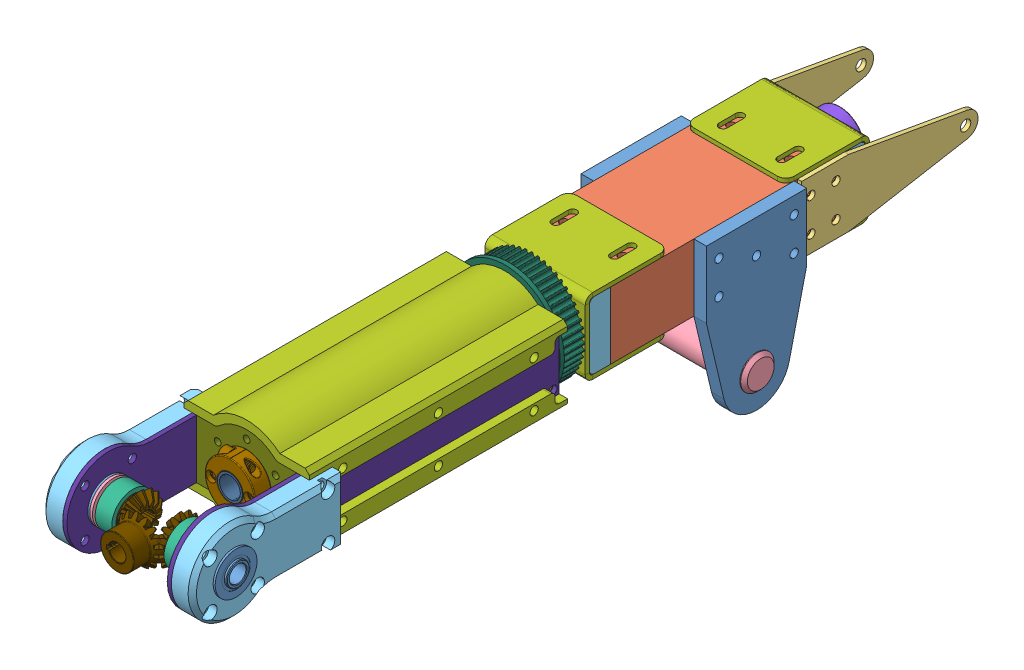
SolidWorks assembly Forearm, configuration Default. Lengths in mm.
Overall size (139.65 143.63 612.78).
45 component instances, 25 part files, 35 mates.
Components (placement in the parent):
- SidePlate^Forearm-1: SidePlate^Forearm [Default] at origin size (47.62 127 76.2) (virtual)
- SidePlate^Forearm-2: SidePlate^Forearm [Default] x (-1 0 0) z (0 0 -1) size (47.62 127 76.2) (virtual)
- Box^Forearm-1: Box^Forearm [Default] at origin size (76.2 50.8 177.8) (virtual)
- BackSidePlate^Forearm-1: BackSidePlate^Forearm [Default] at origin size (41.27 50.8 177.23) (virtual)
- BackSidePlate^Forearm-2: BackSidePlate^Forearm [Default] at (79.375 0 0) size (41.27 50.8 177.23) (virtual)
- 6061K602_HARDENED PRECISION STEEL SHAFT-1: 6061K602_HARDENED PRECISION STEEL SHAFT [6061K602] at (0 609.075 0) size (101.6 25.4 25.4)
- BearingSpacer^Forearm-1: BearingSpacer^Forearm [Default] at origin size (76.2 50.8 22.22) (virtual)
- 6384K367_BALL BEARING-1: 6384K367_BALL BEARING [6384K367] at (0 685.275 115.824) x (1 0 0) z (0 0 -1) size (44.45 44.45 14.3)
- BearingHolder^Forearm-1: BearingHolder^Forearm [Default] at origin size (76.2 57.15 63.5) (virtual)
- BearingSpacer^Forearm-2: BearingSpacer^Forearm [Default] at (0 0 25.4) x (-1 0 0) z (0 0 -1) size (76.2 50.8 22.22) (virtual)
- BearingHolder^Forearm-2: BearingHolder^Forearm [Default] at (0 0 25.4) x (-1 0 0) z (0 0 -1) size (76.2 57.15 63.5) (virtual)
- 6384K367_BALL BEARING-2: 6384K367_BALL BEARING [6384K367] at (0 685.275 -90.424) x (-1 0 0) z (0 0 1) size (44.45 44.45 14.3)
- 6435K160_ONE-PIECE CLAMP-ON SHAFT COLLAR-1: 6435K160_ONE-PIECE CLAMP-ON SHAFT COLLAR [6435K16] at (0 685.275 -104.7242) x (1 0 0) z (0 0 -1) size (38.1 38.11 12.77)
- 9677T100_CLAMP-ON SHAFT COLLAR WITH MOUNTING HOLES-1: 9677T100_CLAMP-ON SHAFT COLLAR WITH MOUNTING HOLES [9677T1] at (0 685.275 159.4517) x (0 -1 0) z (0 0 -1) size (38.14 38.1 13.27)
- 89955K599_Tube^Forearm-1: 89955K599_Tube^Forearm [Default] at origin size (19.05 19.05 463.5) (virtual)
- ThrustBase^Forearm-1: ThrustBase^Forearm [Default] at origin size (44.45 44.45 8.27) (virtual)
- 5909K460_THRUST NEEDLE-ROLLER BEARING-1: 5909K460_THRUST NEEDLE-ROLLER BEARING [5909K46] at (0 685.275 131.2545) x (0 0 -1) z (1 0 0) size (0.81 31.75 31.75)
- 5909K330_THRUST NEEDLE-ROLLER BEARING-1: 5909K330_THRUST NEEDLE-ROLLER BEARING [5909K33] at (0 685.275 132.2467) x (1 0 0) z (0 1 0) size (31.75 1.98 31.75)
- 5909K460_THRUST NEEDLE-ROLLER BEARING-2: 5909K460_THRUST NEEDLE-ROLLER BEARING [5909K46] at (0 685.275 134.0517) x (0 0 -1) z (1 0 0) size (0.81 31.75 31.75)
- PulleySupportPlate^Forearm-1: PulleySupportPlate^Forearm [Default] at origin size (63.5 63.5 3.17) (virtual)
- J4Pulley-1: J4Pulley [Default] at (0 685.275 140.4017) x (-1 0 0) z (0 -1 0) size (84.06 20.68 84.06)
- WristBase^Forearm-1: WristBase^Forearm [Default] at origin size (76.2 63.5 9.53) (virtual)
- WristSidePlate^Forearm-1: WristSidePlate^Forearm [Default] at origin size (3.17 63.5 441.32) (virtual)
- WristSidePlate^Forearm-2: WristSidePlate^Forearm [Default] at (79.375 0 0) size (3.17 63.5 441.32) (virtual)
- WristBase^Forearm-2: WristBase^Forearm [Default] at (0 0 186.6233) size (76.2 63.5 9.53) (virtual)
- 9677T100_CLAMP-ON SHAFT COLLAR WITH MOUNTING HOLES-2: 9677T100_CLAMP-ON SHAFT COLLAR WITH MOUNTING HOLES [9677T1] at (0 685.275 346.075) x (0 -1 0) z (0 0 -1) size (38.14 38.1 13.27)
- 6843K130_MTL MITER GEAR--20 DEG PRESSURE ANGLE-1: 6843K130_MTL MITER GEAR--20 DEG PRESSURE ANGLE [6843K13] at (-31.1638 641.133 394.588) x (0 -0.999847 0.017483) z (0 0.017483 0.999847) size (34.68 21.82 34.5)
- 6843K130_MTL MITER GEAR--20 DEG PRESSURE ANGLE-3: 6843K130_MTL MITER GEAR--20 DEG PRESSURE ANGLE [6843K13] at (-11.812 641.133 437.5638) x (0.017483 -0.999847 0) z (0.999847 0.017483 0) size (34.68 21.82 34.5)
- 6384K361_BALL BEARING-1-1: 6384K361_BALL BEARING-1 [6384K361] at (-41.3385 685.275 406.4) x (0 0 1) z (-1 0 0) size (31.75 31.75 11.13)
- 5909K440_THRUST NEEDLE-ROLLER BEARING-1: 5909K440_THRUST NEEDLE-ROLLER BEARING [5909K44] at (-34.5472 685.275 406.4) size (0.81 23.81 23.81)
- 5909K310_THRUST NEEDLE-ROLLER BEARING-1: 5909K310_THRUST NEEDLE-ROLLER BEARING [5909K31] at (-32.7422 685.275 406.4) x (0 1 0) z (0 0 1) size (23.81 1.98 23.81)
- SideMiterSpacer^Forearm-1: SideMiterSpacer^Forearm [Default] at origin size (2.03 31.75 31.75) (virtual)
- SidePrintedSupport^Forearm-1: SidePrintedSupport^Forearm [Default] at origin size (16.21 63.5 115.89) (virtual)
- 6384K361_BALL BEARING-1-2: 6384K361_BALL BEARING-1 [6384K361] at (-53.9115 685.275 406.4) x (0 0 1) z (1 0 0) size (31.75 31.75 11.13)
- SidePrintedSupport^Forearm-2: SidePrintedSupport^Forearm [Default] at (0 1370.55 0) x (-1 0 0) z (0 0 1) size (16.21 63.5 115.89) (virtual)
- 6384K361_BALL BEARING-1-3: 6384K361_BALL BEARING-1 [6384K361] at (53.9115 685.275 406.4) x (0 0 -1) z (-1 0 0) size (31.75 31.75 11.13)
- 6384K361_BALL BEARING-1-4: 6384K361_BALL BEARING-1 [6384K361] at (41.3385 685.275 406.4) x (0 0 -1) z (1 0 0) size (31.75 31.75 11.13)
- SideMiterSpacer^Forearm-2: SideMiterSpacer^Forearm [Default] at (0 0 812.8) x (-1 0 0) z (0 0 -1) size (2.03 31.75 31.75) (virtual)
- 5909K440_THRUST NEEDLE-ROLLER BEARING-2: 5909K440_THRUST NEEDLE-ROLLER BEARING [5909K44] at (34.5472 685.275 406.4) x (-1 0 0) z (0 0 -1) size (0.81 23.81 23.81)
- 5909K310_THRUST NEEDLE-ROLLER BEARING-2: 5909K310_THRUST NEEDLE-ROLLER BEARING [5909K31] at (32.7422 685.275 406.4) x (0 1 0) z (0 0 1) size (23.81 1.98 23.81)
- 6843K130_MTL MITER GEAR--20 DEG PRESSURE ANGLE-4: 6843K130_MTL MITER GEAR--20 DEG PRESSURE ANGLE [6843K13] at (31.1638 728.9771 393.052) x (0 0.999847 -0.017483) z (0 0.017483 0.999847) size (34.68 21.82 34.5)
- 6391K281_OIL-EMBEDDED SLEEVE BEARING-1: 6391K281_OIL-EMBEDDED SLEEVE BEARING [6391K281] at (-26.162 685.275 406.4) x (0 0 1) z (-1 0 0) size (31.78 31.78 12.7)
- 6391K281_OIL-EMBEDDED SLEEVE BEARING-2: 6391K281_OIL-EMBEDDED SLEEVE BEARING [6391K281] at (26.162 685.275 406.4) x (0 0 1) z (-1 0 0) size (31.78 31.78 12.7)
- WristCover^Forearm-1: WristCover^Forearm [Default] at origin size (95.25 25.4 196.15) (virtual)
- WristCover^Forearm-2: WristCover^Forearm [Default] at (0 1370.55 0) x (-1 0 0) z (0 0 1) size (95.25 25.4 196.15) (virtual)
Mates (geometry in assembly coordinates):
- Concentric1: concentric anti-aligned: cylinder of SidePlate^Forearm-1 through (-47.625 609.075 0) axis (1 0 0) radius 12.7; circle of 6061K602_HARDENED PRECISION STEEL SHAFT-1
- Width1: width anti-aligned: plane of 6061K602_HARDENED PRECISION STEEL SHAFT-1 through (-50.8 609.075 0) normal (-1 0 0); plane of SidePlate^Forearm-2 through (50.8 609.075 0) normal (1 0 0); plane of 6061K602_HARDENED PRECISION STEEL SHAFT-1 through (47.625 609.075 0) normal (1 0 0); plane of SidePlate^Forearm-1 through (-47.625 609.075 0) normal (-1 0 0)
- Concentric2: concentric aligned: cylinder of 6384K367_BALL BEARING-1 through (0 685.275 109.474) axis (0 0 -1) radius 20.6375; cylinder of BearingHolder^Forearm-1 through (0 685.275 120.65) axis (0 0 -1) radius 20.6375
- Coincident2: coincident anti-aligned: plane of 6384K367_BALL BEARING-1 through (0 669.8646 120.65) normal (0 0 -1); plane of BearingHolder^Forearm-1 through (0 0 120.65) normal (0 0 1)
- Concentric3: concentric aligned: cylinder of 6384K367_BALL BEARING-2 through (0 685.275 -84.074) axis (0 0 1) radius 9.525; cylinder of 6435K160_ONE-PIECE CLAMP-ON SHAFT COLLAR-1 through (0 685.275 -111.0742) axis (0 0 1) radius 9.525
- Coincident3: coincident anti-aligned: plane of 6384K367_BALL BEARING-2 through (0 674.4038 -98.3742) normal (0 0 -1); plane of 6435K160_ONE-PIECE CLAMP-ON SHAFT COLLAR-1 through (0 685.275 -98.3742) normal (0 0 1)
- Concentric4: concentric anti-aligned: cylinder of 6384K367_BALL BEARING-1 through (0 685.275 109.474) axis (0 0 -1) radius 9.525; cylinder of 9677T100_CLAMP-ON SHAFT COLLAR WITH MOUNTING HOLES-1 through (0 685.275 153.1017) axis (0 0 1) radius 9.525
- Concentric5: concentric anti-aligned: cylinder of 89955K599_Tube^Forearm-1 through (0 685.275 379.3658) axis (0 0 -1) radius 9.525; cylinder of 5909K460_THRUST NEEDLE-ROLLER BEARING-1 through (0 685.275 130.4417) axis (0 0 1) radius 9.5504
- Coincident4: coincident anti-aligned: plane of ThrustBase^Forearm-1 through (0 685.275 130.4417) normal (0 0 1); plane of 5909K460_THRUST NEEDLE-ROLLER BEARING-1 through (0 685.275 130.4417) normal (0 0 -1)
- Concentric6: concentric anti-aligned: cylinder of 89955K599_Tube^Forearm-1 through (0 685.275 379.3658) axis (0 0 -1) radius 9.525; cylinder of 5909K330_THRUST NEEDLE-ROLLER BEARING-1 through (0 685.275 133.2389) axis (0 0 1) radius 9.5504
- Tangent1: tangent anti-aligned: plane of 5909K460_THRUST NEEDLE-ROLLER BEARING-1 through (0 685.275 131.2545) normal (0 0 1); cylinder of 5909K330_THRUST NEEDLE-ROLLER BEARING-1 through (-5.4469 671.5178 132.2467) axis (-0.368125 -0.929776 0) radius 0.9922
- Concentric7: concentric anti-aligned: cylinder of 89955K599_Tube^Forearm-1 through (0 685.275 379.3658) axis (0 0 -1) radius 9.525; cylinder of 5909K460_THRUST NEEDLE-ROLLER BEARING-2 through (0 685.275 133.2389) axis (0 0 1) radius 9.5504
- Tangent2: tangent anti-aligned: cylinder of 5909K330_THRUST NEEDLE-ROLLER BEARING-1 through (-1.8545 670.5954 132.2467) axis (-0.125333 -0.992115 0) radius 0.9922; plane of 5909K460_THRUST NEEDLE-ROLLER BEARING-2 through (0 685.275 133.2389) normal (0 0 -1)
- Concentric8: concentric anti-aligned: cylinder of 89955K599_Tube^Forearm-1 through (0 685.275 379.3658) axis (0 0 -1) radius 9.525; circle of J4Pulley-1
- Coincident6: coincident anti-aligned: plane of PulleySupportPlate^Forearm-1 through (0 0 137.2267) normal (0 0 1); plane of J4Pulley-1 through (0 685.275 137.2267) normal (0 0 -1)
- Parallel1: parallel anti-aligned: plane of 9677T100_CLAMP-ON SHAFT COLLAR WITH MOUNTING HOLES-1 through (0.0953 704.3248 153.1017) normal (-1 0 0)
- Coincident11: coincident anti-aligned: plane of 9677T100_CLAMP-ON SHAFT COLLAR WITH MOUNTING HOLES-1 through (0 685.275 153.1017) normal (0 0 -1); plane of WristBase^Forearm-1 through (-24.5934 712.2625 153.1017) normal (0 0 1)
- Concentric10: concentric aligned: cylinder of 89955K599_Tube^Forearm-1 through (0 685.275 379.3658) axis (0 0 -1) radius 9.525; cylinder of WristBase^Forearm-2 through (0 685.275 339.725) axis (0 0 -1) radius 9.525
- Distance2: distance = 330.2 mm: plane of assembly through (0 0 0) normal (0 0 1); plane of assembly; plane of WristBase^Forearm-2 through (-24.5934 712.2625 330.2) normal (0 0 -1)
- Concentric11: concentric anti-aligned: cylinder of 89955K599_Tube^Forearm-1 through (0 685.275 379.3658) axis (0 0 -1) radius 7.9375; cylinder of 9677T100_CLAMP-ON SHAFT COLLAR WITH MOUNTING HOLES-2 through (0 685.275 339.725) axis (0 0 1) radius 9.525
- Coincident13: coincident anti-aligned: plane of WristBase^Forearm-2 through (-24.5934 712.2625 339.725) normal (0 0 1); plane of 9677T100_CLAMP-ON SHAFT COLLAR WITH MOUNTING HOLES-2 through (0 685.275 339.725) normal (0 0 -1)
- Concentric12: concentric anti-aligned: cylinder of WristSidePlate^Forearm-1 through (-41.275 685.275 406.4) axis (1 0 0) radius 14.2875; cylinder of 6843K130_MTL MITER GEAR--20 DEG PRESSURE ANGLE-1 through (31.0355 685.275 406.4) axis (-1 0 0) radius 6.3563
- Concentric13: concentric anti-aligned: cylinder of 89955K599_Tube^Forearm-1 through (0 685.275 379.3658) axis (0 0 -1) radius 7.9375; cylinder of 6843K130_MTL MITER GEAR--20 DEG PRESSURE ANGLE-3 through (0 685.275 375.3645) axis (0 0 1) radius 6.3563
- Distance3: distance = 31.75 mm: cylinder of 6843K130_MTL MITER GEAR--20 DEG PRESSURE ANGLE-3 through (0 685.275 375.3645) axis (0 0 1) radius 6.3563; plane of 6843K130_MTL MITER GEAR--20 DEG PRESSURE ANGLE-1 through (-31.75 685.053 393.7019) normal (-1 0 0)
- Distance4: distance = 31.75 mm: plane of 6843K130_MTL MITER GEAR--20 DEG PRESSURE ANGLE-3 through (-12.6981 685.053 438.15) normal (0 0 1); cylinder of 6843K130_MTL MITER GEAR--20 DEG PRESSURE ANGLE-1 through (31.0355 685.275 406.4) axis (-1 0 0) radius 6.3563
- Concentric14: concentric anti-aligned: cylinder of WristSidePlate^Forearm-1 through (-41.275 685.275 406.4) axis (1 0 0) radius 14.2875; cylinder of 6384K361_BALL BEARING-1-1 through (-46.101 685.275 406.4) axis (-1 0 0) radius 14.2875
- Coincident14: coincident anti-aligned: plane of WristSidePlate^Forearm-1 through (-38.1 637.65 374.8091) normal (1 0 0); plane of 6384K361_BALL BEARING-1-1 through (-38.1 695.9938 406.4) normal (-1 0 0)
- Concentric15: concentric aligned: cylinder of 6843K130_MTL MITER GEAR--20 DEG PRESSURE ANGLE-1 through (31.0355 685.275 406.4) axis (-1 0 0) radius 6.3563; cylinder of 5909K440_THRUST NEEDLE-ROLLER BEARING-1 through (-33.7344 685.275 406.4) axis (-1 0 0) radius 6.3754
- Concentric16: concentric anti-aligned: cylinder of 6843K130_MTL MITER GEAR--20 DEG PRESSURE ANGLE-1 through (31.0355 685.275 406.4) axis (-1 0 0) radius 6.3563; cylinder of 5909K310_THRUST NEEDLE-ROLLER BEARING-1 through (-31.75 685.275 406.4) axis (1 0 0) radius 6.3754
- Tangent6: tangent anti-aligned: plane of 6843K130_MTL MITER GEAR--20 DEG PRESSURE ANGLE-1 through (-31.75 685.053 393.7019) normal (-1 0 0); cylinder of 5909K310_THRUST NEEDLE-ROLLER BEARING-1 through (-32.7422 674.394 409.1554) axis (0 -0.9694 0.245485) radius 0.9922
- Tangent7: tangent anti-aligned: plane of 5909K440_THRUST NEEDLE-ROLLER BEARING-1 through (-33.7344 685.275 406.4) normal (1 0 0); cylinder of 5909K310_THRUST NEEDLE-ROLLER BEARING-1 through (-32.7422 674.394 409.1554) axis (0 -0.9694 0.245485) radius 0.9922
- Concentric17: concentric aligned: cylinder of SidePrintedSupport^Forearm-1 through (-57.15 685.275 406.4) axis (1 0 0) radius 14.2875; cylinder of 6384K361_BALL BEARING-1-2 through (-49.149 685.275 406.4) axis (1 0 0) radius 14.2875
- Coincident16: coincident anti-aligned: plane of SidePrintedSupport^Forearm-1 through (-57.15 0 0) normal (-1 0 0); plane of 6384K361_BALL BEARING-1-2 through (-57.15 674.5562 406.4) normal (1 0 0)
- Concentric18: concentric anti-aligned: cylinder of 6843K130_MTL MITER GEAR--20 DEG PRESSURE ANGLE-1 through (31.0355 685.275 406.4) axis (-1 0 0) radius 12.7; cylinder of 6391K281_OIL-EMBEDDED SLEEVE BEARING-1 through (-32.512 685.275 406.4) axis (1 0 0) radius 12.7
- Distance5: distance = 5.588 mm anti-aligned: plane of WristSidePlate^Forearm-1 through (-38.1 637.65 374.8091) normal (1 0 0); plane of 6391K281_OIL-EMBEDDED SLEEVE BEARING-1 through (-32.512 685.275 406.4) normal (-1 0 0)
